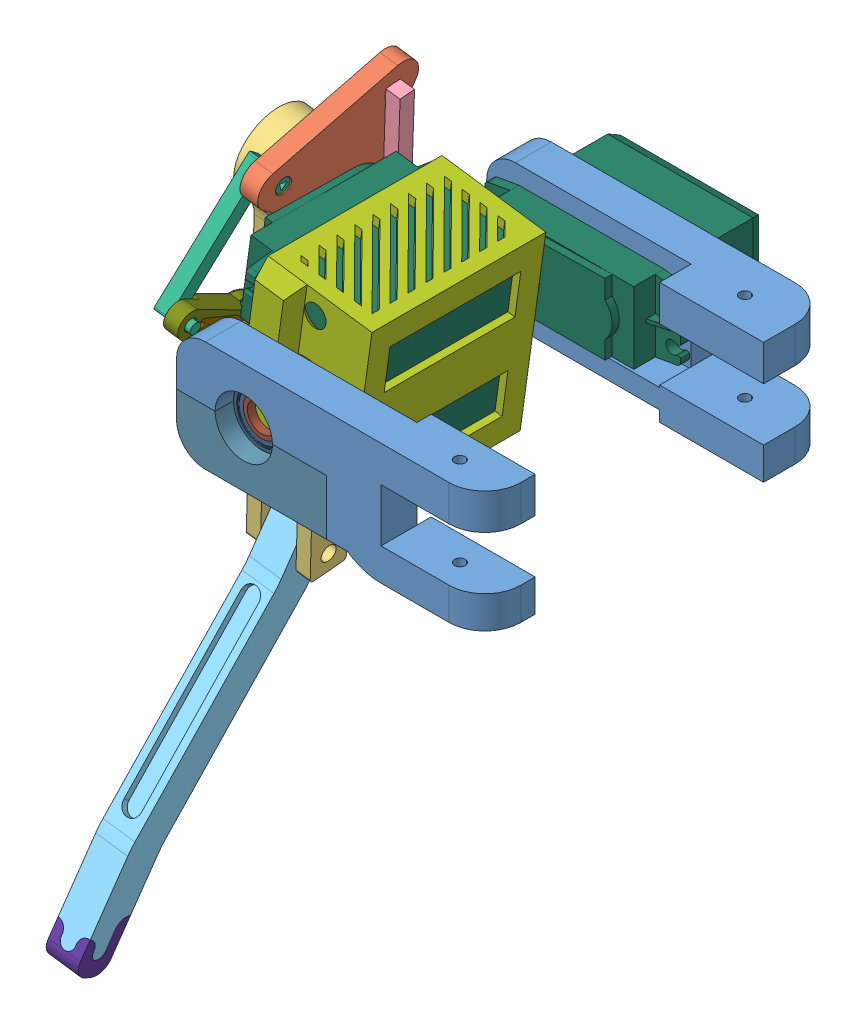
SolidWorks assembly Reverse Robot Assembly, configuration Default. Lengths in mm.
Overall size (132.79 216.88 113.75).
30 component instances, 17 part files, 39 mates.
Components (placement in the parent):
- RearLegMount-1: RearLegMount [Default] at (-158.0372 73.3871 37.3879) size (86 33.8 96.5)
- RearRotatingPiece-1: RearRotatingPiece [Default] at (-38.0357 72.1303 81.9379) x (-0.137616 -0.990307 0.018825) z (0.002591 0.018646 0.999823) size (44.28 6 43.21)
- RearUpperLeg-1: RearUpperLeg [Default] at (-53.6067 -30.4762 65.161) x (0.015479 0.111391 -0.993656) z (0.990482 -0.13764 0) size (22 116.4 18)
- RearLongConnectingRod-1: RearLongConnectingRod [Default] at (-86.6094 103.2886 73.0357) x (-0.014587 -0.104968 0.994369) z (-0.136865 -0.984905 -0.105976) size (5 22 107.31)
- RearLowerLeg-1: RearLowerLeg [Default] at (-60.2529 -110.9973 125.9197) x (0.057307 0.412391 0.909203) z (-0.990482 0.13764 0) size (20.21 126 9.59)
- RearShortConnectingRod-1: RearShortConnectingRod [Default] at (-34.6566 58.6673 123.3169) x (0.108188 0.77854 -0.618199) z (0.990482 -0.13764 0) size (37.08 4 13)
- RearServoHousing-2: RearServoHousing [Default] at (-41.658 118.7173 92.4379) x (0 0 1) z (-0.990482 0.13764 0) size (61.5 52 29.25)
- Circle Rudder-1: Circle Rudder [默认] at (-33.2872 57.9871 65.1879) x (-0.854749 -0.519042 0) z (0.519042 -0.854749 0) size (20.8 5.5 20.8)
- Double_Blade_Rudder-1: Double_Blade_Rudder [默认] at (-66.9694 49.1844 102.9379) x (-0.10901 -0.784459 0.610525) z (0.084033 0.604714 0.791997) size (12.2 5.5 38)
- 688ZZ Bearing Assembly-1: 688ZZ Bearing Assembly [Default] at (-33.2872 57.9871 126.3879) size (17.99 17.98 5)
  - Outer Ring-1: Outer Ring [Default] at origin size (16 16 5)
  - Inner Ring-1: Inner Ring [Default] x (-0.241565 -0.970385 0) z (0 0 1) size (10.6 10.6 5)
  - Cage-1: Cage [Default] x (0.535517 0.844524 0) z (0 0 1) size (13.01 13.06 2.21)
  - 2mm Ball Bearing-1: 2mm Ball Bearing [Default] at (-5.0671 3.2131 0) x (0.050652 0.835774 0.546732) z (0.977207 -0.154478 0.145614) size (2 2 2)
  - 2mm Ball Bearing-2: 2mm Ball Bearing [Default] at (-5.988 -0.3789 0) x (-0.450278 0.705928 0.546732) z (0.881377 0.449412 0.145614) size (2 2 2)
  - 2mm Ball Bearing-3: 2mm Ball Bearing [Default] at (-4.6217 -3.8262 0) x (-0.779216 0.306441 0.546732) z (0.448891 0.881642 0.145614) size (2 2 2)
  - 2mm Ball Bearing-4: 2mm Ball Bearing [Default] at (-1.49 -5.812 0) x (-0.810521 -0.210096 0.546732) z (-0.155056 0.977115 0.145614) size (2 2 2)
  - 2mm Ball Bearing-5: 2mm Ball Bearing [Default] at (2.2108 -5.5778 0) x (-0.532234 -0.646383 0.546732) z (-0.699777 0.699363 0.145614) size (2 2 2)
  - 2mm Ball Bearing-6: 2mm Ball Bearing [Default] at (5.0671 -3.2131 0) x (-0.050652 -0.835774 0.546732) z (-0.977207 0.154478 0.145614) size (2 2 2)
  - 2mm Ball Bearing-7: 2mm Ball Bearing [Default] at (5.988 0.3789 0) x (0.450278 -0.705928 0.546732) z (-0.881377 -0.449412 0.145614) size (2 2 2)
  - 2mm Ball Bearing-8: 2mm Ball Bearing [Default] at (4.6217 3.8262 0) x (0.779216 -0.306441 0.546732) z (-0.448891 -0.881642 0.145614) size (2 2 2)
  - 2mm Ball Bearing-9: 2mm Ball Bearing [Default] at (1.49 5.812 0) x (0.810521 0.210096 0.546732) z (0.155056 -0.977115 0.145614) size (2 2 2)
  - 2mm Ball Bearing-10: 2mm Ball Bearing [Default] at (-2.2108 5.5778 0) x (0.532234 0.646383 0.546732) z (0.699777 -0.699363 0.145614) size (2 2 2)
- Lower Leg Mount-1: Lower Leg Mount [Default] at (-52.0372 57.9871 133.8879) x (-1 0 0) z (0 0 -1) size (41.75 15.4 10)
- MG996R-3: MG996R [Default] at (-22.7872 58.4435 20.1379) x (1 0 0) z (0 -1 0) size (54.5 42.75 20)
- Circle Rudder-2: Circle Rudder [默认] at (-63.0949 75.6126 81.9379) x (-0.120143 -0.864571 0.487937) z (0.06716 0.483293 0.872879) size (20.8 5.5 20.8)
- MG996R-4: MG996R [Default] at (-22.164 42.8558 92.4379) x (0 0 -1) z (0.13764 0.990482 0) size (54.5 42.75 20)
- MG996R-5: MG996R [Default] at (-18.4598 69.5123 92.4379) x (0 0 1) z (-0.13764 -0.990482 0) size (54.5 42.75 20)
- Servo Arm Mount-1: Servo Arm Mount [Default] at (-67.0685 49.1981 102.9379) x (-0.10901 -0.784459 0.610525) z (-0.990482 0.13764 0) size (16.2 34.39 7.06)
- Foot Cap-1: Foot Cap [Default] at (-87.7979 -98.5219 110.9987) x (0.057307 0.412391 0.909203) z (-0.990482 0.13764 0) size (10.5 14 9.53)
Mates (geometry in assembly coordinates):
- Coincident6: coincident anti-aligned: plane of RearLegMount-1 through (-25.2872 57.9871 123.8879) normal (0 -1 0); plane of Lower Leg Mount-1 through (-25.2872 57.9871 123.8879) normal (0 1 0)
- Coincident7: coincident anti-aligned: plane of RearLegMount-1 through (-10.2872 57.9871 123.8879) normal (-1 0 0); plane of Lower Leg Mount-1 through (-10.2872 57.9871 123.8879) normal (1 0 0)
- Coincident8: coincident aligned: plane of RearLegMount-1 through (33.9628 73.3871 133.8879) normal (0 0 1); plane of Lower Leg Mount-1 through (-33.2872 57.9871 133.8879) normal (0 0 1)
- Concentric3: concentric anti-aligned: cylinder of RearLegMount-1 through (-33.2872 57.9871 133.8879) axis (0 0 -1) radius 8; cylinder of 688ZZ Bearing Assembly-1/Outer Ring-1 through (-33.2872 57.9871 133.1433) axis (0 0 1) radius 8
- Coincident9: coincident aligned: plane of RearLegMount-1 through (-52.0372 -28.6129 123.8879) normal (0 0 -1); plane of 688ZZ Bearing Assembly-1/Outer Ring-1 through (-33.2872 64.9871 123.8879) normal (0 0 -1)
- Concentric4: concentric anti-aligned: cylinder of 688ZZ Bearing Assembly-1/Inner Ring-1 through (-33.2872 57.9871 133.1433) axis (0 0 1) radius 4; cylinder of RearServoHousing-2 through (-33.2872 57.9871 156.4252) axis (0 0 -1) radius 4
- Concentric5: concentric anti-aligned: circle of RearLegMount-1; cylinder of MG996R-3 through (-47.7872 53.2153 47.3879) axis (0 0 1) radius 1.7678
- Concentric6: concentric anti-aligned: circle of RearLegMount-1; cylinder of MG996R-3 through (-47.7872 63.2153 47.3879) axis (0 0 1) radius 1.7678
- Coincident12: coincident anti-aligned: plane of RearLegMount-1 through (-52.0372 -28.6129 47.3879) normal (0 0 1); plane of MG996R-3 through (-47.7872 63.2153 47.3879) normal (0 0 -1)
- Concentric7: concentric anti-aligned: circle of Circle Rudder-1; circle of RearServoHousing-2
- Coincident15: coincident anti-aligned: plane of RearServoHousing-2 through (56.0881 58.6922 94.9252) normal (0 0 -1); plane of Circle Rudder-1 through (-35.9131 58.8771 68.3879) normal (0 0 1)
- Concentric8: concentric aligned: cylinder of MG996R-5 through (-44.7936 77.9894 97.1752) axis (-0.990482 0.13764 0) radius 1.7678; cylinder of RearServoHousing-2 through (-36.8698 76.8883 97.1752) axis (-0.990482 0.13764 0) radius 0.7
- Coincident16: coincident anti-aligned: plane of RearServoHousing-2 through (-18.5226 69.0603 122.1752) normal (-0.990482 0.13764 0); plane of MG996R-5 through (-18.4598 69.5123 122.1752) normal (0.990482 -0.13764 0)
- Concentric9: concentric anti-aligned: cylinder of MG996R-5 through (-46.17 68.0846 147.1752) axis (-0.990482 0.13764 0) radius 1.7678; circle of RearServoHousing-2
- Concentric10: concentric anti-aligned: cylinder of MG996R-4 through (-48.4351 51.7849 147.1752) axis (-0.990482 0.13764 0) radius 1.7678; circle of RearServoHousing-2
- Coincident17: coincident anti-aligned: plane of RearServoHousing-2 through (-18.5226 69.0603 122.1752) normal (-0.990482 0.13764 0); plane of MG996R-4 through (-22.164 42.8558 122.1752) normal (0.990482 -0.13764 0)
- Parallel2: parallel anti-aligned: plane of MG996R-4 through (-58.9502 37.8716 142.4252) normal (-0.13764 -0.990482 0); plane of RearServoHousing-2 through (51.1331 23.0349 122.1752) normal (0.13764 0.990482 0)
- Concentric12: concentric aligned: cylinder of Circle Rudder-2 through (-60.8168 75.296 111.6752) axis (-0.990482 0.13764 0) radius 1.5; cylinder of MG996R-5 through (-57.8454 74.8831 111.6752) axis (-0.990482 0.13764 0) radius 1.5
- Coincident20: coincident anti-aligned: plane of Circle Rudder-2 through (-60.8168 75.296 111.6752) normal (0.990482 -0.13764 0); plane of MG996R-5 through (-60.8168 75.296 111.6752) normal (-0.990482 0.13764 0)
- Coincident21: coincident anti-aligned: plane of RearUpperLeg-1 through (-63.0949 75.6126 111.6752) normal (0.990482 -0.13764 0); plane of Circle Rudder-2 through (-63.0949 75.6126 111.6752) normal (-0.990482 0.13764 0)
- Concentric13: concentric anti-aligned: cylinder of RearUpperLeg-1 through (-72.0093 76.8514 111.6752) axis (0.990482 -0.13764 0) radius 1.7; cylinder of Circle Rudder-2 through (-60.8168 75.296 111.6752) axis (-0.990482 0.13764 0) radius 1.5
- Concentric14: concentric anti-aligned: cylinder of RearRotatingPiece-1 through (-59.8264 75.1584 111.6752) axis (0.990482 -0.13764 0) radius 4.5; cylinder of Circle Rudder-2 through (-57.6473 74.8556 111.6752) axis (-0.990482 0.13764 0) radius 4.4
- Coincident22: coincident anti-aligned: plane of RearRotatingPiece-1 through (-57.8454 74.8831 111.6752) normal (0.990482 -0.13764 0); plane of MG996R-5 through (-57.8454 74.8831 111.6752) normal (-0.990482 0.13764 0)
- Concentric16: concentric aligned: cylinder of Double_Blade_Rudder-1 through (-64.6913 48.8678 132.6752) axis (-0.990482 0.13764 0) radius 1.5; cylinder of MG996R-4 through (-61.5218 48.4273 132.6752) axis (-0.990482 0.13764 0) radius 1.5
- Coincident24: coincident anti-aligned: plane of Double_Blade_Rudder-1 through (-61.5218 48.4273 132.6752) normal (0.990482 -0.13764 0); plane of MG996R-4 through (-61.5218 48.4273 132.6752) normal (-0.990482 0.13764 0)
- Coincident25: coincident anti-aligned: plane of Double_Blade_Rudder-1 through (-66.9694 49.1844 132.6752) normal (-0.990482 0.13764 0); plane of Servo Arm Mount-1 through (-66.9694 49.1844 132.6752) normal (0.990482 -0.13764 0)
- Concentric17: concentric aligned: cylinder of Double_Blade_Rudder-1 through (-64.6913 48.8678 132.6752) axis (-0.990482 0.13764 0) radius 1.5; cylinder of Servo Arm Mount-1 through (-66.9694 49.1844 132.6752) axis (-0.990482 0.13764 0) radius 1.6
- Concentric18: concentric anti-aligned: cylinder of RearRotatingPiece-1 through (-60.602 91.3726 127.6551) axis (0.990482 -0.13764 0) radius 2.2; cylinder of RearShortConnectingRod-1 through (-55.8477 90.7119 127.6551) axis (-0.990482 0.13764 0) radius 2
- Concentric19: concentric aligned: cylinder of RearShortConnectingRod-1 through (-59.4762 64.6006 148.2935) axis (-0.990482 0.13764 0) radius 1.5; cylinder of Servo Arm Mount-1 through (-60.8629 64.7933 148.2935) axis (-0.990482 0.13764 0) radius 1.7
- Coincident27: coincident anti-aligned: plane of RearShortConnectingRod-1 through (-64.8177 65.3951 150.7929) normal (0.990482 -0.13764 0); plane of Servo Arm Mount-1 through (-67.0685 49.1981 132.6752) normal (-0.990482 0.13764 0)
- Concentric23: concentric aligned: cylinder of RearUpperLeg-1 through (-71.7995 -16.0884 71.5224) axis (-0.990482 0.13764 0) radius 2.1; cylinder of RearLowerLeg-1 through (-76.2567 -15.469 71.5224) axis (-0.990482 0.13764 0) radius 2
- Distance3: distance = 0.5 mm anti-aligned: plane of RearLowerLeg-1 through (-97.8912 -105.767 125.9197) normal (-0.990482 0.13764 0); plane of RearUpperLeg-1 through (-87.5308 -27.5787 81.0595) normal (0.990482 -0.13764 0)
- Concentric24: concentric anti-aligned: cylinder of RearRotatingPiece-1 through (-59.9774 95.8671 97.353) axis (0.990482 -0.13764 0) radius 2.2; cylinder of RearLongConnectingRod-1 through (-61.166 96.0323 97.353) axis (-0.990482 0.13764 0) radius 2
- Concentric25: concentric anti-aligned: cylinder of RearLongConnectingRod-1 through (-81.5211 6.2227 57.5943) axis (0.990482 -0.13764 0) radius 2; cylinder of RearLowerLeg-1 through (-73.3992 5.0941 57.5943) axis (-0.990482 0.13764 0) radius 2.1
- Coincident30: coincident anti-aligned: plane of RearLongConnectingRod-1 through (-54.8819 96.209 99.9833) normal (-0.990482 0.13764 0); plane of RearRotatingPiece-1 through (-57.8454 74.8831 111.6752) normal (0.990482 -0.13764 0)
- Concentric26: concentric aligned: cylinder of RearLowerLeg-1 through (-90.0626 -82.1247 129.1325) axis (-0.076683 -0.551825 -0.830427) radius 2; cylinder of Foot Cap-1 through (-89.6792 -79.3656 133.2846) axis (-0.076683 -0.551825 -0.830427) radius 2
- Concentric27: concentric aligned: cylinder of RearLowerLeg-1 through (-95.1484 -86.0292 132.1967) axis (0.990482 -0.13764 0) radius 2; cylinder of Foot Cap-1 through (-95.1484 -86.0292 132.1967) axis (0.990482 -0.13764 0) radius 2
- Concentric28: concentric aligned: cylinder of Double_Blade_Rudder-1 through (-63.3993 58.1653 141.669) axis (-0.990482 0.13764 0) radius 0.75; cylinder of Servo Arm Mount-1 through (-65.6774 58.4819 141.669) axis (-0.990482 0.13764 0) radius 0.75
- Coincident31: coincident anti-aligned: plane of Circle Rudder-1 through (-33.2872 57.9871 62.8879) normal (0 0 -1); plane of MG996R-3 through (-33.2872 58.3421 62.8879) normal (0 0 1)
